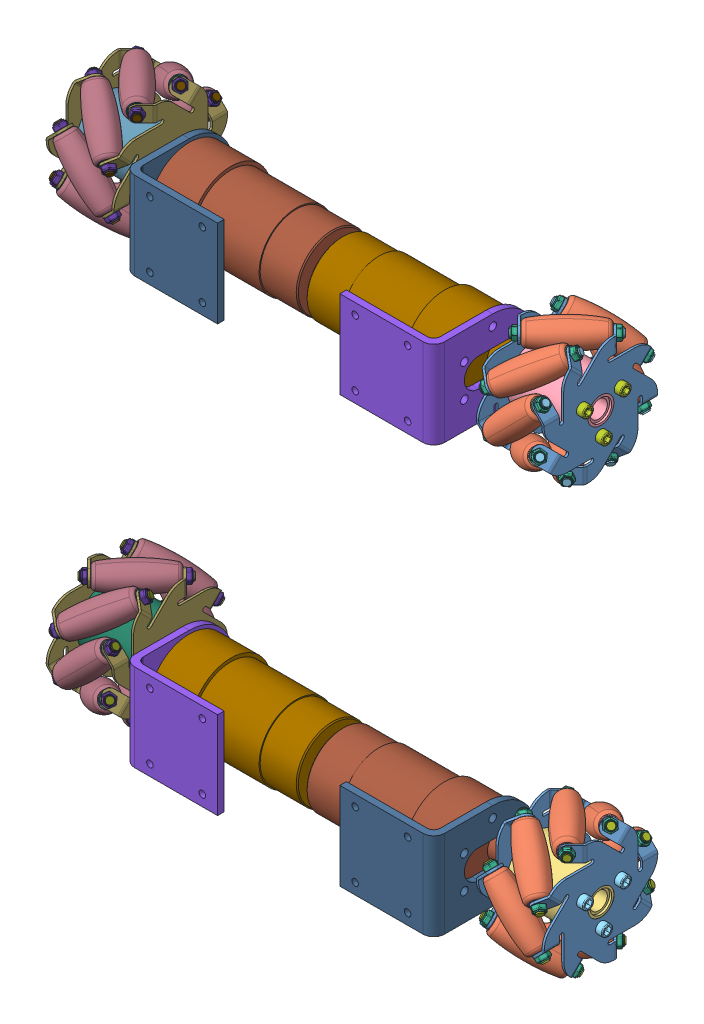
SolidWorks assembly car, configuration 默认. Lengths in mm.
Overall size (280 281.77 89.29).
257 component instances, 48 part files, 0 mates.
Components (placement in the parent):
- Tank(2)^car-1: Tank(2)^car [默认] at origin size (280 382.88 170.83) (virtual)
  - Mecanum_Wheel_60mm_Right_ASM_AP214 v1^Tank(2)_car-1: Mecanum_Wheel_60mm_Right_ASM_AP214 v1^Tank(2)_car [默认] at (62.5 -23.5276 -89.1195) x (1 0 0) z (0 0 -1) size (83 63.25 63.25) (virtual)
    - plate_2_Varsayilan^Mecanum_Wheel_60mm_Right_ASM_AP214 v1_Tank(2)_car-1: plate_2_Varsayilan^Mecanum_Wheel_60mm_Right_ASM_AP214 v1_Tank(2)_car [默认] at (56.8037 4.8798 97.2247) x (0.707107 0.707107 0) z (0 0 1) size (41.63 41.63 53.77) (virtual)
    - roller_Varsayilan^Mecanum_Wheel_60mm_Right_ASM_AP214 v1_Tank(2)_car-1: roller_Varsayilan^Mecanum_Wheel_60mm_Right_ASM_AP214 v1_Tank(2)_car [默认] at (15.1622 40.0059 51.0708) x (-0.707107 0.5 0.5) z (-0.704237 -0.434326 -0.561615) size (29.8 12.94 12.94) (virtual)
    - liner_Varsayilan^Mecanum_Wheel_60mm_Right_ASM_AP214 v1_Tank(2)_car-1: liner_Varsayilan^Mecanum_Wheel_60mm_Right_ASM_AP214 v1_Tank(2)_car [默认] at (4.8906 47.2689 58.3339) x (-0.663539 -0.224823 -0.713562) z (-0.24437 -0.836334 0.490743) size (7 1 7) (virtual)
    - inner_cylinder_Varsayilan^Mecanum_Wheel_60mm_Right_ASM_AP214 v1_Tank(2)_car-1: inner_cylinder_Varsayilan^Mecanum_Wheel_60mm_Right_ASM_AP214 v1_Tank(2)_car [默认] at (30 23.5276 67.1195) x (0 0 1) z (-1 0 0) size (26 26 31) (virtual)
    - two_sided_screw_Varsayilan^Mecanum_Wheel_60mm_Right_ASM_AP214 v1_Tank(2)_car-1: two_sided_screw_Varsayilan^Mecanum_Wheel_60mm_Right_ASM_AP214 v1_Tank(2)_car [默认] at (28.9323 30.2689 41.3339) x (-0.195015 0.541787 -0.817579) z (-0.707107 0.5 0.5) size (3 3 38) (virtual)
    - 3mm_bolt_Varsayilan^Mecanum_Wheel_60mm_Right_ASM_AP214 v1_Tank(2)_car-1: 3mm_bolt_Varsayilan^Mecanum_Wheel_60mm_Right_ASM_AP214 v1_Tank(2)_car [默认] at (4.155 47.7891 58.854) x (0.638071 0.755922 0.146447) z (-0.707107 0.5 0.5) size (5.6 5.2 2.5) (virtual)
    - 3x35_screw_Varsayilan^Mecanum_Wheel_60mm_Right_ASM_AP214 v1_Tank(2)_car-1: 3x35_screw_Varsayilan^Mecanum_Wheel_60mm_Right_ASM_AP214 v1_Tank(2)_car [默认] at (-3 18.5276 58.4592) x (0 0.745603 -0.666391) z (1 0 0) size (5 5 37) (virtual)
    - plate_2_Varsayilan^Mecanum_Wheel_60mm_Right_ASM_AP214 v1_Tank(2)_car-2: plate_2_Varsayilan^Mecanum_Wheel_60mm_Right_ASM_AP214 v1_Tank(2)_car [默认] at (-25.8037 4.8798 37.0142) x (-0.707107 0.707107 0) z (0 0 -1) size (41.63 41.63 53.77) (virtual)
    - liner_Varsayilan^Mecanum_Wheel_60mm_Right_ASM_AP214 v1_Tank(2)_car-2: liner_Varsayilan^Mecanum_Wheel_60mm_Right_ASM_AP214 v1_Tank(2)_car [默认] at (26.1038 32.2689 43.3339) x (0.54662 -0.062042 0.835079) z (-0.448561 -0.8638 0.22944) size (7 1 7) (virtual)
    - 3mm_bolt_Varsayilan^Mecanum_Wheel_60mm_Right_ASM_AP214 v1_Tank(2)_car-2: 3mm_bolt_Varsayilan^Mecanum_Wheel_60mm_Right_ASM_AP214 v1_Tank(2)_car [默认] at (26.8109 31.7689 42.8339) x (0.358192 -0.356391 0.862951) z (0.707107 -0.5 -0.5) size (5.6 5.2 2.5) (virtual)
    - 3mm_bolt_Varsayilan^Mecanum_Wheel_60mm_Right_ASM_AP214 v1_Tank(2)_car-3: 3mm_bolt_Varsayilan^Mecanum_Wheel_60mm_Right_ASM_AP214 v1_Tank(2)_car [默认] at (0 18.5276 75.7797) x (0 -0.80734 0.590087) z (-1 0 0) size (5.6 5.2 2.5) (virtual)
    - 3x35_screw_Varsayilan^Mecanum_Wheel_60mm_Right_ASM_AP214 v1_Tank(2)_car-2: 3x35_screw_Varsayilan^Mecanum_Wheel_60mm_Right_ASM_AP214 v1_Tank(2)_car [默认] at (-3 18.5276 75.7797) x (0 -0.949913 -0.312516) z (1 0 0) size (5 5 37) (virtual)
    - 3x35_screw_Varsayilan^Mecanum_Wheel_60mm_Right_ASM_AP214 v1_Tank(2)_car-3: 3x35_screw_Varsayilan^Mecanum_Wheel_60mm_Right_ASM_AP214 v1_Tank(2)_car [默认] at (-3 33.5276 67.1195) x (0 0.20431 0.978906) z (1 0 0) size (5 5 37) (virtual)
    - 3mm_bolt_Varsayilan^Mecanum_Wheel_60mm_Right_ASM_AP214 v1_Tank(2)_car-4: 3mm_bolt_Varsayilan^Mecanum_Wheel_60mm_Right_ASM_AP214 v1_Tank(2)_car [默认] at (0 33.5276 67.1195) x (0 0.9147 0.404133) z (-1 0 0) size (5.6 5.2 2.5) (virtual)
    - 3mm_bolt_Varsayilan^Mecanum_Wheel_60mm_Right_ASM_AP214 v1_Tank(2)_car-5: 3mm_bolt_Varsayilan^Mecanum_Wheel_60mm_Right_ASM_AP214 v1_Tank(2)_car [默认] at (0 18.5276 58.4592) x (0 -0.107361 -0.99422) z (-1 0 0) size (5.6 5.2 2.5) (virtual)
    - two_sided_screw_Varsayilan^Mecanum_Wheel_60mm_Right_ASM_AP214 v1_Tank(2)_car-2: two_sided_screw_Varsayilan^Mecanum_Wheel_60mm_Right_ASM_AP214 v1_Tank(2)_car [默认] at (28.9323 10.0613 44.1195) x (-0.195015 -0.195015 -0.961217) z (-0.707107 0.707107 0) size (3 3 38) (virtual)
    - two_sided_screw_Varsayilan^Mecanum_Wheel_60mm_Right_ASM_AP214 v1_Tank(2)_car-3: two_sided_screw_Varsayilan^Mecanum_Wheel_60mm_Right_ASM_AP214 v1_Tank(2)_car [默认] at (28.9323 -2.258 60.3781) x (-0.195015 -0.817579 -0.541787) z (-0.707107 0.5 -0.5) size (3 3 38) (virtual)
    - two_sided_screw_Varsayilan^Mecanum_Wheel_60mm_Right_ASM_AP214 v1_Tank(2)_car-4: two_sided_screw_Varsayilan^Mecanum_Wheel_60mm_Right_ASM_AP214 v1_Tank(2)_car [默认] at (28.9323 0.5276 80.5857) x (-0.195015 -0.961217 0.195015) z (-0.707107 0 -0.707107) size (3 3 38) (virtual)
    - two_sided_screw_Varsayilan^Mecanum_Wheel_60mm_Right_ASM_AP214 v1_Tank(2)_car-5: two_sided_screw_Varsayilan^Mecanum_Wheel_60mm_Right_ASM_AP214 v1_Tank(2)_car [默认] at (28.9323 16.7862 92.905) x (-0.195015 -0.541787 0.817579) z (-0.707107 -0.5 -0.5) size (3 3 38) (virtual)
    - two_sided_screw_Varsayilan^Mecanum_Wheel_60mm_Right_ASM_AP214 v1_Tank(2)_car-6: two_sided_screw_Varsayilan^Mecanum_Wheel_60mm_Right_ASM_AP214 v1_Tank(2)_car [默认] at (28.9323 36.9938 90.1195) x (-0.195015 0.195015 0.961217) z (-0.707107 -0.707107 0) size (3 3 38) (virtual)
    - two_sided_screw_Varsayilan^Mecanum_Wheel_60mm_Right_ASM_AP214 v1_Tank(2)_car-7: two_sided_screw_Varsayilan^Mecanum_Wheel_60mm_Right_ASM_AP214 v1_Tank(2)_car [默认] at (28.9323 49.3131 73.8608) x (-0.195015 0.817579 0.541787) z (-0.707107 -0.5 0.5) size (3 3 38) (virtual)
    - two_sided_screw_Varsayilan^Mecanum_Wheel_60mm_Right_ASM_AP214 v1_Tank(2)_car-8: two_sided_screw_Varsayilan^Mecanum_Wheel_60mm_Right_ASM_AP214 v1_Tank(2)_car [默认] at (28.9323 46.5276 53.6532) x (-0.195015 0.961217 -0.195015) z (-0.707107 0 0.707107) size (3 3 38) (virtual)
    - 3mm_bolt_Varsayilan^Mecanum_Wheel_60mm_Right_ASM_AP214 v1_Tank(2)_car-6: 3mm_bolt_Varsayilan^Mecanum_Wheel_60mm_Right_ASM_AP214 v1_Tank(2)_car [默认] at (26.8109 12.1826 44.1195) x (0.358192 0.358192 0.862205) z (0.707107 -0.707107 0) size (5.6 5.2 2.5) (virtual)
    - 3mm_bolt_Varsayilan^Mecanum_Wheel_60mm_Right_ASM_AP214 v1_Tank(2)_car-7: 3mm_bolt_Varsayilan^Mecanum_Wheel_60mm_Right_ASM_AP214 v1_Tank(2)_car [默认] at (26.8109 -0.758 58.8781) x (0.358192 0.862951 0.356391) z (0.707107 -0.5 0.5) size (5.6 5.2 2.5) (virtual)
    - 3mm_bolt_Varsayilan^Mecanum_Wheel_60mm_Right_ASM_AP214 v1_Tank(2)_car-8: 3mm_bolt_Varsayilan^Mecanum_Wheel_60mm_Right_ASM_AP214 v1_Tank(2)_car [默认] at (26.8109 0.5276 78.4644) x (0.358192 0.862205 -0.358192) z (0.707107 0 0.707107) size (5.6 5.2 2.5) (virtual)
    - 3mm_bolt_Varsayilan^Mecanum_Wheel_60mm_Right_ASM_AP214 v1_Tank(2)_car-9: 3mm_bolt_Varsayilan^Mecanum_Wheel_60mm_Right_ASM_AP214 v1_Tank(2)_car [默认] at (26.8109 15.2862 91.405) x (0.358192 0.356391 -0.862951) z (0.707107 0.5 0.5) size (5.6 5.2 2.5) (virtual)
    - 3mm_bolt_Varsayilan^Mecanum_Wheel_60mm_Right_ASM_AP214 v1_Tank(2)_car-10: 3mm_bolt_Varsayilan^Mecanum_Wheel_60mm_Right_ASM_AP214 v1_Tank(2)_car [默认] at (26.8109 34.8725 90.1195) x (0.358192 -0.358192 -0.862205) z (0.707107 0.707107 0) size (5.6 5.2 2.5) (virtual)
    - 3mm_bolt_Varsayilan^Mecanum_Wheel_60mm_Right_ASM_AP214 v1_Tank(2)_car-11: 3mm_bolt_Varsayilan^Mecanum_Wheel_60mm_Right_ASM_AP214 v1_Tank(2)_car [默认] at (26.8109 47.8131 75.3608) x (0.358192 -0.862951 -0.356391) z (0.707107 0.5 -0.5) size (5.6 5.2 2.5) (virtual)
    - 3mm_bolt_Varsayilan^Mecanum_Wheel_60mm_Right_ASM_AP214 v1_Tank(2)_car-12: 3mm_bolt_Varsayilan^Mecanum_Wheel_60mm_Right_ASM_AP214 v1_Tank(2)_car [默认] at (26.8109 46.5276 55.7745) x (0.358192 -0.862205 0.358192) z (0.707107 0 -0.707107) size (5.6 5.2 2.5) (virtual)
    - 3mm_bolt_Varsayilan^Mecanum_Wheel_60mm_Right_ASM_AP214 v1_Tank(2)_car-13: 3mm_bolt_Varsayilan^Mecanum_Wheel_60mm_Right_ASM_AP214 v1_Tank(2)_car [默认] at (4.155 34.8385 44.1195) x (0.638071 0.638071 -0.430964) z (-0.707107 0.707107 0) size (5.6 5.2 2.5) (virtual)
    - 3mm_bolt_Varsayilan^Mecanum_Wheel_60mm_Right_ASM_AP214 v1_Tank(2)_car-14: 3mm_bolt_Varsayilan^Mecanum_Wheel_60mm_Right_ASM_AP214 v1_Tank(2)_car [默认] at (4.155 15.2622 42.858) x (0.638071 0.146447 -0.755922) z (-0.707107 0.5 -0.5) size (5.6 5.2 2.5) (virtual)
    - 3mm_bolt_Varsayilan^Mecanum_Wheel_60mm_Right_ASM_AP214 v1_Tank(2)_car-15: 3mm_bolt_Varsayilan^Mecanum_Wheel_60mm_Right_ASM_AP214 v1_Tank(2)_car [默认] at (4.155 0.5276 55.8085) x (0.638071 -0.430964 -0.638071) z (-0.707107 0 -0.707107) size (5.6 5.2 2.5) (virtual)
    - 3mm_bolt_Varsayilan^Mecanum_Wheel_60mm_Right_ASM_AP214 v1_Tank(2)_car-16: 3mm_bolt_Varsayilan^Mecanum_Wheel_60mm_Right_ASM_AP214 v1_Tank(2)_car [默认] at (4.155 -0.7339 75.3849) x (0.638071 -0.755922 -0.146447) z (-0.707107 -0.5 -0.5) size (5.6 5.2 2.5) (virtual)
    - 3mm_bolt_Varsayilan^Mecanum_Wheel_60mm_Right_ASM_AP214 v1_Tank(2)_car-17: 3mm_bolt_Varsayilan^Mecanum_Wheel_60mm_Right_ASM_AP214 v1_Tank(2)_car [默认] at (4.155 12.2166 90.1195) x (0.638071 -0.638071 0.430964) z (-0.707107 -0.707107 0) size (5.6 5.2 2.5) (virtual)
    - 3mm_bolt_Varsayilan^Mecanum_Wheel_60mm_Right_ASM_AP214 v1_Tank(2)_car-18: 3mm_bolt_Varsayilan^Mecanum_Wheel_60mm_Right_ASM_AP214 v1_Tank(2)_car [默认] at (4.155 31.793 91.381) x (0.638071 -0.146447 0.755922) z (-0.707107 -0.5 0.5) size (5.6 5.2 2.5) (virtual)
    - 3mm_bolt_Varsayilan^Mecanum_Wheel_60mm_Right_ASM_AP214 v1_Tank(2)_car-19: 3mm_bolt_Varsayilan^Mecanum_Wheel_60mm_Right_ASM_AP214 v1_Tank(2)_car [默认] at (4.155 46.5276 78.4304) x (0.638071 0.430964 0.638071) z (-0.707107 0 0.707107) size (5.6 5.2 2.5) (virtual)
    - liner_Varsayilan^Mecanum_Wheel_60mm_Right_ASM_AP214 v1_Tank(2)_car-3: liner_Varsayilan^Mecanum_Wheel_60mm_Right_ASM_AP214 v1_Tank(2)_car [默认] at (26.1038 12.8897 44.1195) x (0.54662 0.54662 0.634361) z (-0.448561 -0.448561 0.773037) size (7 1 7) (virtual)
    - liner_Varsayilan^Mecanum_Wheel_60mm_Right_ASM_AP214 v1_Tank(2)_car-4: liner_Varsayilan^Mecanum_Wheel_60mm_Right_ASM_AP214 v1_Tank(2)_car [默认] at (26.1038 -0.258 58.3781) x (0.54662 0.835079 0.062042) z (-0.448561 0.22944 0.8638) size (7 1 7) (virtual)
    - liner_Varsayilan^Mecanum_Wheel_60mm_Right_ASM_AP214 v1_Tank(2)_car-5: liner_Varsayilan^Mecanum_Wheel_60mm_Right_ASM_AP214 v1_Tank(2)_car [默认] at (26.1038 0.5276 77.7573) x (0.54662 0.634361 -0.54662) z (-0.448561 0.773037 0.448561) size (7 1 7) (virtual)
    - liner_Varsayilan^Mecanum_Wheel_60mm_Right_ASM_AP214 v1_Tank(2)_car-6: liner_Varsayilan^Mecanum_Wheel_60mm_Right_ASM_AP214 v1_Tank(2)_car [默认] at (26.1038 14.7862 90.905) x (0.54662 0.062042 -0.835079) z (-0.448561 0.8638 -0.22944) size (7 1 7) (virtual)
    - liner_Varsayilan^Mecanum_Wheel_60mm_Right_ASM_AP214 v1_Tank(2)_car-7: liner_Varsayilan^Mecanum_Wheel_60mm_Right_ASM_AP214 v1_Tank(2)_car [默认] at (26.1038 34.1654 90.1195) x (0.54662 -0.54662 -0.634361) z (-0.448561 0.448561 -0.773037) size (7 1 7) (virtual)
    - liner_Varsayilan^Mecanum_Wheel_60mm_Right_ASM_AP214 v1_Tank(2)_car-8: liner_Varsayilan^Mecanum_Wheel_60mm_Right_ASM_AP214 v1_Tank(2)_car [默认] at (26.1038 47.3131 75.8608) x (0.54662 -0.835079 -0.062042) z (-0.448561 -0.22944 -0.8638) size (7 1 7) (virtual)
    - liner_Varsayilan^Mecanum_Wheel_60mm_Right_ASM_AP214 v1_Tank(2)_car-9: liner_Varsayilan^Mecanum_Wheel_60mm_Right_ASM_AP214 v1_Tank(2)_car [默认] at (26.1038 46.5276 56.4816) x (0.54662 -0.634361 0.54662) z (-0.448561 -0.773037 -0.448561) size (7 1 7) (virtual)
    - liner_Varsayilan^Mecanum_Wheel_60mm_Right_ASM_AP214 v1_Tank(2)_car-10: liner_Varsayilan^Mecanum_Wheel_60mm_Right_ASM_AP214 v1_Tank(2)_car [默认] at (4.8906 34.1029 44.1195) x (-0.663539 -0.663539 -0.345591) z (-0.24437 -0.24437 0.938385) size (7 1 7) (virtual)
    - liner_Varsayilan^Mecanum_Wheel_60mm_Right_ASM_AP214 v1_Tank(2)_car-11: liner_Varsayilan^Mecanum_Wheel_60mm_Right_ASM_AP214 v1_Tank(2)_car [默认] at (4.8906 14.742 43.3781) x (-0.663539 -0.713562 0.224823) z (-0.24437 0.490743 0.836334) size (7 1 7) (virtual)
    - liner_Varsayilan^Mecanum_Wheel_60mm_Right_ASM_AP214 v1_Tank(2)_car-12: liner_Varsayilan^Mecanum_Wheel_60mm_Right_ASM_AP214 v1_Tank(2)_car [默认] at (4.8906 0.5276 56.5441) x (-0.663539 -0.345591 0.663539) z (-0.24437 0.938385 0.24437) size (7 1 7) (virtual)
    - liner_Varsayilan^Mecanum_Wheel_60mm_Right_ASM_AP214 v1_Tank(2)_car-13: liner_Varsayilan^Mecanum_Wheel_60mm_Right_ASM_AP214 v1_Tank(2)_car [默认] at (4.8906 -0.2138 75.905) x (-0.663539 0.224823 0.713562) z (-0.24437 0.836334 -0.490743) size (7 1 7) (virtual)
    - liner_Varsayilan^Mecanum_Wheel_60mm_Right_ASM_AP214 v1_Tank(2)_car-14: liner_Varsayilan^Mecanum_Wheel_60mm_Right_ASM_AP214 v1_Tank(2)_car [默认] at (4.8906 12.9522 90.1195) x (-0.663539 0.663539 0.345591) z (-0.24437 0.24437 -0.938385) size (7 1 7) (virtual)
    - liner_Varsayilan^Mecanum_Wheel_60mm_Right_ASM_AP214 v1_Tank(2)_car-15: liner_Varsayilan^Mecanum_Wheel_60mm_Right_ASM_AP214 v1_Tank(2)_car [默认] at (4.8906 32.3131 90.8608) x (-0.663539 0.713562 -0.224823) z (-0.24437 -0.490743 -0.836334) size (7 1 7) (virtual)
    - liner_Varsayilan^Mecanum_Wheel_60mm_Right_ASM_AP214 v1_Tank(2)_car-16: liner_Varsayilan^Mecanum_Wheel_60mm_Right_ASM_AP214 v1_Tank(2)_car [默认] at (4.8906 46.5276 77.6948) x (-0.663539 0.345591 -0.663539) z (-0.24437 -0.938385 -0.24437) size (7 1 7) (virtual)
    - roller_Varsayilan^Mecanum_Wheel_60mm_Right_ASM_AP214 v1_Tank(2)_car-2: roller_Varsayilan^Mecanum_Wheel_60mm_Right_ASM_AP214 v1_Tank(2)_car [默认] at (15.1622 23.8314 44.1195) x (-0.707107 0.707107 0) z (-0.704237 -0.704237 -0.090007) size (29.8 12.94 12.94) (virtual)
    - roller_Varsayilan^Mecanum_Wheel_60mm_Right_ASM_AP214 v1_Tank(2)_car-3: roller_Varsayilan^Mecanum_Wheel_60mm_Right_ASM_AP214 v1_Tank(2)_car [默认] at (15.1622 7.4789 50.6412) x (-0.707107 0.5 -0.5) z (-0.704237 -0.561615 0.434326) size (29.8 12.94 12.94) (virtual)
    - roller_Varsayilan^Mecanum_Wheel_60mm_Right_ASM_AP214 v1_Tank(2)_car-4: roller_Varsayilan^Mecanum_Wheel_60mm_Right_ASM_AP214 v1_Tank(2)_car [默认] at (15.1622 0.5276 66.8156) x (-0.707107 0 -0.707107) z (-0.704237 -0.090007 0.704237) size (29.8 12.94 12.94) (virtual)
    - roller_Varsayilan^Mecanum_Wheel_60mm_Right_ASM_AP214 v1_Tank(2)_car-5: roller_Varsayilan^Mecanum_Wheel_60mm_Right_ASM_AP214 v1_Tank(2)_car [默认] at (15.1622 7.0493 83.1681) x (-0.707107 -0.5 -0.5) z (-0.704237 0.434326 0.561615) size (29.8 12.94 12.94) (virtual)
    - roller_Varsayilan^Mecanum_Wheel_60mm_Right_ASM_AP214 v1_Tank(2)_car-6: roller_Varsayilan^Mecanum_Wheel_60mm_Right_ASM_AP214 v1_Tank(2)_car [默认] at (15.1622 23.2237 90.1195) x (-0.707107 -0.707107 0) z (-0.704237 0.704237 0.090007) size (29.8 12.94 12.94) (virtual)
    - roller_Varsayilan^Mecanum_Wheel_60mm_Right_ASM_AP214 v1_Tank(2)_car-7: roller_Varsayilan^Mecanum_Wheel_60mm_Right_ASM_AP214 v1_Tank(2)_car [默认] at (15.1622 39.5762 83.5977) x (-0.707107 -0.5 0.5) z (-0.704237 0.561615 -0.434326) size (29.8 12.94 12.94) (virtual)
    - roller_Varsayilan^Mecanum_Wheel_60mm_Right_ASM_AP214 v1_Tank(2)_car-8: roller_Varsayilan^Mecanum_Wheel_60mm_Right_ASM_AP214 v1_Tank(2)_car [默认] at (15.1622 46.5276 67.4233) x (-0.707107 0 0.707107) z (-0.704237 0.090007 -0.704237) size (29.8 12.94 12.94) (virtual)
  - DC RF^Tank(2)_car-1: DC RF^Tank(2)_car [默认] at (0 -47.0551 -178.2389) x (1 0 0) z (0 0 -1) size (95 40 47) (virtual)
    - Component10^DC RF_Tank(2)_car-1: Component10^DC RF_Tank(2)_car [默认] at origin size (43 40 47) (virtual)
    - DC RF-0^DC RF_Tank(2)_car-1: DC RF-0^DC RF_Tank(2)_car [默认] at origin size (95 37 37) (virtual)
  - DC LF^Tank(2)_car-1: DC LF^Tank(2)_car [默认] at (-41 -47.0551 -178.2389) x (-1 0 0) z (0 0 1) size (95 40 47) (virtual)
    - Component10(Mirror)^DC LF_Tank(2)_car-1: Component10(Mirror)^DC LF_Tank(2)_car [默认] at origin size (43 40 47) (virtual)
    - DC LF-1^DC LF_Tank(2)_car-1: DC LF-1^DC LF_Tank(2)_car [默认] at origin size (95 37 37) (virtual)
  - Mecanum_Wheel_60mm_Left_ASM_AP214 v1^Tank(2)_car-1: Mecanum_Wheel_60mm_Left_ASM_AP214 v1^Tank(2)_car [默认] at (-107.4753 -26.4281 -134.5883) x (1 0 0) z (0 -0.707107 -0.707107) size (37 63.14 63.14) (virtual)
    - plate_1_Varsayilan^Mecanum_Wheel_60mm_Left_ASM_AP214 v1_Tank(2)_car-1: plate_1_Varsayilan^Mecanum_Wheel_60mm_Left_ASM_AP214 v1_Tank(2)_car [默认] at (-26.0247 -30.9199 60) size (7.04 53.75 53.75) (virtual)
    - roller_Varsayilan (1)^Mecanum_Wheel_60mm_Left_ASM_AP214 v1_Tank(2)_car-1: roller_Varsayilan (1)^Mecanum_Wheel_60mm_Left_ASM_AP214 v1_Tank(2)_car [默认] at (-11.1205 15.2872 46.4107) x (0.707107 -0.5 0.5) z (-0.228848 -0.830871 -0.50723) size (29.8 12.94 12.94) (virtual)
    - inner_cylinder_Varsayilan (1)^Mecanum_Wheel_60mm_Left_ASM_AP214 v1_Tank(2)_car-1: inner_cylinder_Varsayilan (1)^Mecanum_Wheel_60mm_Left_ASM_AP214 v1_Tank(2)_car [默认] at (-26.0247 -0.7238 29.8948) x (0 0.707107 -0.707107) z (1 0 0) size (26 26 31) (virtual)
    - liner_Varsayilan (1)^Mecanum_Wheel_60mm_Left_ASM_AP214 v1_Tank(2)_car-1: liner_Varsayilan (1)^Mecanum_Wheel_60mm_Left_ASM_AP214 v1_Tank(2)_car [默认] at (-0.849 8.0242 53.6738) x (0.666667 0.707107 -0.235702) z (-0.235702 0.5 0.833333) size (7 1 7) (virtual)
    - 3x35_screw_Varsayilan (1)^Mecanum_Wheel_60mm_Left_ASM_AP214 v1_Tank(2)_car-1: 3x35_screw_Varsayilan (1)^Mecanum_Wheel_60mm_Left_ASM_AP214 v1_Tank(2)_car [默认] at (-29.9304 6.3473 36.9659) x (0 0 -1) z (1 0 0) size (5 5 37) (virtual)
    - 3mm_bolt_Varsayilan (1)^Mecanum_Wheel_60mm_Left_ASM_AP214 v1_Tank(2)_car-1: 3mm_bolt_Varsayilan (1)^Mecanum_Wheel_60mm_Left_ASM_AP214 v1_Tank(2)_car [默认] at (-27.0247 1.8644 20.2355) x (0 0.765139 -0.643866) z (-1 0 0) size (5.6 5.2 2.5) (virtual)
    - two_sided_screw_Varsayilan (1)^Mecanum_Wheel_60mm_Left_ASM_AP214 v1_Tank(2)_car-1: two_sided_screw_Varsayilan (1)^Mecanum_Wheel_60mm_Left_ASM_AP214 v1_Tank(2)_car [默认] at (-24.8906 6.0552 4.1469) x (-0.576606 0.817021 -0.001578) z (0.707107 0.5 0.5) size (3 3 38) (virtual)
    - plate_1_Varsayilan^Mecanum_Wheel_60mm_Left_ASM_AP214 v1_Tank(2)_car-2: plate_1_Varsayilan^Mecanum_Wheel_60mm_Left_ASM_AP214 v1_Tank(2)_car [默认] at (3.0696 29.3814 -0.3013) x (-1 0 0) z (0 1 0) size (7.04 53.75 53.75) (virtual)
    - liner_Varsayilan (1)^Mecanum_Wheel_60mm_Left_ASM_AP214 v1_Tank(2)_car-2: liner_Varsayilan (1)^Mecanum_Wheel_60mm_Left_ASM_AP214 v1_Tank(2)_car [默认] at (-22.0622 23.0242 38.6738) x (0 -0.707107 -0.707107) z (-0.707107 -0.5 0.5) size (7 1 7) (virtual)
    - liner_Varsayilan (1)^Mecanum_Wheel_60mm_Left_ASM_AP214 v1_Tank(2)_car-3: liner_Varsayilan (1)^Mecanum_Wheel_60mm_Left_ASM_AP214 v1_Tank(2)_car [默认] at (-22.0622 22.2762 19.3102) x (0 -1 0) z (-0.707107 0 0.707107) size (7 1 7) (virtual)
    - liner_Varsayilan (1)^Mecanum_Wheel_60mm_Left_ASM_AP214 v1_Tank(2)_car-4: liner_Varsayilan (1)^Mecanum_Wheel_60mm_Left_ASM_AP214 v1_Tank(2)_car [默认] at (-22.0622 8.0552 6.1469) x (0 -0.707107 0.707107) z (-0.707107 0.5 0.5) size (7 1 7) (virtual)
    - liner_Varsayilan (1)^Mecanum_Wheel_60mm_Left_ASM_AP214 v1_Tank(2)_car-5: liner_Varsayilan (1)^Mecanum_Wheel_60mm_Left_ASM_AP214 v1_Tank(2)_car [默认] at (-22.0622 -11.3084 6.8948) x (0 0 1) z (-0.707107 0.707107 0) size (7 1 7) (virtual)
    - liner_Varsayilan (1)^Mecanum_Wheel_60mm_Left_ASM_AP214 v1_Tank(2)_car-6: liner_Varsayilan (1)^Mecanum_Wheel_60mm_Left_ASM_AP214 v1_Tank(2)_car [默认] at (-22.0622 -24.4717 21.1158) x (0 0.707107 0.707107) z (-0.707107 0.5 -0.5) size (7 1 7) (virtual)
    - liner_Varsayilan (1)^Mecanum_Wheel_60mm_Left_ASM_AP214 v1_Tank(2)_car-7: liner_Varsayilan (1)^Mecanum_Wheel_60mm_Left_ASM_AP214 v1_Tank(2)_car [默认] at (-22.0622 -23.7238 40.4794) x (0 1 0) z (-0.707107 0 -0.707107) size (7 1 7) (virtual)
    - liner_Varsayilan (1)^Mecanum_Wheel_60mm_Left_ASM_AP214 v1_Tank(2)_car-8: liner_Varsayilan (1)^Mecanum_Wheel_60mm_Left_ASM_AP214 v1_Tank(2)_car [默认] at (-22.0622 -9.5028 53.6427) x (0 0.707107 -0.707107) z (-0.707107 -0.5 -0.5) size (7 1 7) (virtual)
    - liner_Varsayilan (1)^Mecanum_Wheel_60mm_Left_ASM_AP214 v1_Tank(2)_car-9: liner_Varsayilan (1)^Mecanum_Wheel_60mm_Left_ASM_AP214 v1_Tank(2)_car [默认] at (-22.0622 9.8609 52.8948) x (0 0 -1) z (-0.707107 -0.707107 0) size (7 1 7) (virtual)
    - liner_Varsayilan (1)^Mecanum_Wheel_60mm_Left_ASM_AP214 v1_Tank(2)_car-10: liner_Varsayilan (1)^Mecanum_Wheel_60mm_Left_ASM_AP214 v1_Tank(2)_car [默认] at (-0.849 22.2762 40.5234) x (0.666667 0.333333 -0.666667) z (-0.235702 0.942809 0.235702) size (7 1 7) (virtual)
    - liner_Varsayilan (1)^Mecanum_Wheel_60mm_Left_ASM_AP214 v1_Tank(2)_car-11: liner_Varsayilan (1)^Mecanum_Wheel_60mm_Left_ASM_AP214 v1_Tank(2)_car [默认] at (-0.849 23.0552 21.1469) x (0.666667 -0.235702 -0.707107) z (-0.235702 0.833333 -0.5) size (7 1 7) (virtual)
    - liner_Varsayilan (1)^Mecanum_Wheel_60mm_Left_ASM_AP214 v1_Tank(2)_car-12: liner_Varsayilan (1)^Mecanum_Wheel_60mm_Left_ASM_AP214 v1_Tank(2)_car [默认] at (-0.849 9.9048 6.8948) x (0.666667 -0.666667 -0.333333) z (-0.235702 0.235702 -0.942809) size (7 1 7) (virtual)
    - liner_Varsayilan (1)^Mecanum_Wheel_60mm_Left_ASM_AP214 v1_Tank(2)_car-13: liner_Varsayilan (1)^Mecanum_Wheel_60mm_Left_ASM_AP214 v1_Tank(2)_car [默认] at (-0.849 -9.4717 6.1158) x (0.666667 -0.707107 0.235702) z (-0.235702 -0.5 -0.833333) size (7 1 7) (virtual)
    - liner_Varsayilan (1)^Mecanum_Wheel_60mm_Left_ASM_AP214 v1_Tank(2)_car-14: liner_Varsayilan (1)^Mecanum_Wheel_60mm_Left_ASM_AP214 v1_Tank(2)_car [默认] at (-0.849 -23.7238 19.2662) x (0.666667 -0.333333 0.666667) z (-0.235702 -0.942809 -0.235702) size (7 1 7) (virtual)
    - liner_Varsayilan (1)^Mecanum_Wheel_60mm_Left_ASM_AP214 v1_Tank(2)_car-15: liner_Varsayilan (1)^Mecanum_Wheel_60mm_Left_ASM_AP214 v1_Tank(2)_car [默认] at (-0.849 -24.5028 38.6427) x (0.666667 0.235702 0.707107) z (-0.235702 -0.833333 0.5) size (7 1 7) (virtual)
    - liner_Varsayilan (1)^Mecanum_Wheel_60mm_Left_ASM_AP214 v1_Tank(2)_car-16: liner_Varsayilan (1)^Mecanum_Wheel_60mm_Left_ASM_AP214 v1_Tank(2)_car [默认] at (-0.849 -11.3523 52.8948) x (0.666667 0.666667 0.333333) z (-0.235702 -0.235702 0.942809) size (7 1 7) (virtual)
    - roller_Varsayilan (1)^Mecanum_Wheel_60mm_Left_ASM_AP214 v1_Tank(2)_car-2: roller_Varsayilan (1)^Mecanum_Wheel_60mm_Left_ASM_AP214 v1_Tank(2)_car [默认] at (-11.1205 22.2762 30.2518) x (0.707107 0 0.707107) z (-0.228848 -0.94618 0.228848) size (29.8 12.94 12.94) (virtual)
    - roller_Varsayilan (1)^Mecanum_Wheel_60mm_Left_ASM_AP214 v1_Tank(2)_car-3: roller_Varsayilan (1)^Mecanum_Wheel_60mm_Left_ASM_AP214 v1_Tank(2)_car [默认] at (-11.1205 15.7922 13.8838) x (0.707107 0.5 0.5) z (-0.228848 -0.50723 0.830871) size (29.8 12.94 12.94) (virtual)
    - roller_Varsayilan (1)^Mecanum_Wheel_60mm_Left_ASM_AP214 v1_Tank(2)_car-4: roller_Varsayilan (1)^Mecanum_Wheel_60mm_Left_ASM_AP214 v1_Tank(2)_car [默认] at (-11.1205 -0.3667 6.8948) x (0.707107 0.707107 0) z (-0.228848 0.228848 0.94618) size (29.8 12.94 12.94) (virtual)
    - roller_Varsayilan (1)^Mecanum_Wheel_60mm_Left_ASM_AP214 v1_Tank(2)_car-5: roller_Varsayilan (1)^Mecanum_Wheel_60mm_Left_ASM_AP214 v1_Tank(2)_car [默认] at (-11.1205 -16.7348 13.3789) x (0.707107 0.5 -0.5) z (-0.228848 0.830871 0.50723) size (29.8 12.94 12.94) (virtual)
    - roller_Varsayilan (1)^Mecanum_Wheel_60mm_Left_ASM_AP214 v1_Tank(2)_car-6: roller_Varsayilan (1)^Mecanum_Wheel_60mm_Left_ASM_AP214 v1_Tank(2)_car [默认] at (-11.1205 -23.7238 29.5377) x (0.707107 0 -0.707107) z (-0.228848 0.94618 -0.228848) size (29.8 12.94 12.94) (virtual)
    - roller_Varsayilan (1)^Mecanum_Wheel_60mm_Left_ASM_AP214 v1_Tank(2)_car-7: roller_Varsayilan (1)^Mecanum_Wheel_60mm_Left_ASM_AP214 v1_Tank(2)_car [默认] at (-11.1205 -17.2397 45.9058) x (0.707107 -0.5 -0.5) z (-0.228848 0.50723 -0.830871) size (29.8 12.94 12.94) (virtual)
    - roller_Varsayilan (1)^Mecanum_Wheel_60mm_Left_ASM_AP214 v1_Tank(2)_car-8: roller_Varsayilan (1)^Mecanum_Wheel_60mm_Left_ASM_AP214 v1_Tank(2)_car [默认] at (-11.1205 -1.0808 52.8948) x (0.707107 -0.707107 0) z (-0.228848 -0.228848 -0.94618) size (29.8 12.94 12.94) (virtual)
    - 3x35_screw_Varsayilan (1)^Mecanum_Wheel_60mm_Left_ASM_AP214 v1_Tank(2)_car-2: 3x35_screw_Varsayilan (1)^Mecanum_Wheel_60mm_Left_ASM_AP214 v1_Tank(2)_car [默认] at (-29.9304 1.8644 20.2355) x (0 -0.866025 0.5) z (1 0 0) size (5 5 37) (virtual)
    - 3x35_screw_Varsayilan (1)^Mecanum_Wheel_60mm_Left_ASM_AP214 v1_Tank(2)_car-3: 3x35_screw_Varsayilan (1)^Mecanum_Wheel_60mm_Left_ASM_AP214 v1_Tank(2)_car [默认] at (-29.9304 -10.383 32.483) x (0 0.866025 0.5) z (1 0 0) size (5 5 37) (virtual)
    - 3mm_bolt_Varsayilan (1)^Mecanum_Wheel_60mm_Left_ASM_AP214 v1_Tank(2)_car-2: 3mm_bolt_Varsayilan (1)^Mecanum_Wheel_60mm_Left_ASM_AP214 v1_Tank(2)_car [默认] at (-27.0247 -10.383 32.483) x (0 -0.940173 -0.340697) z (-1 0 0) size (5.6 5.2 2.5) (virtual)
    - 3mm_bolt_Varsayilan (1)^Mecanum_Wheel_60mm_Left_ASM_AP214 v1_Tank(2)_car-3: 3mm_bolt_Varsayilan (1)^Mecanum_Wheel_60mm_Left_ASM_AP214 v1_Tank(2)_car [默认] at (-27.0247 6.3473 36.9659) x (0 0.175035 0.984562) z (-1 0 0) size (5.6 5.2 2.5) (virtual)
    - 3mm_bolt_Varsayilan (1)^Mecanum_Wheel_60mm_Left_ASM_AP214 v1_Tank(2)_car-4: 3mm_bolt_Varsayilan (1)^Mecanum_Wheel_60mm_Left_ASM_AP214 v1_Tank(2)_car [默认] at (-22.8133 7.5242 5.6158) x (-0.060636 0.747379 -0.661626) z (-0.707107 -0.5 -0.5) size (5.6 5.2 2.5) (virtual)
    - 3mm_bolt_Varsayilan (1)^Mecanum_Wheel_60mm_Left_ASM_AP214 v1_Tank(2)_car-5: 3mm_bolt_Varsayilan (1)^Mecanum_Wheel_60mm_Left_ASM_AP214 v1_Tank(2)_car [默认] at (-0.1419 23.5552 21.6469) x (0.267213 0.465725 -0.843622) z (0.707107 0.5 0.5) size (5.6 5.2 2.5) (virtual)
    - 3mm_bolt_Varsayilan (1)^Mecanum_Wheel_60mm_Left_ASM_AP214 v1_Tank(2)_car-6: 3mm_bolt_Varsayilan (1)^Mecanum_Wheel_60mm_Left_ASM_AP214 v1_Tank(2)_car [默认] at (-22.8133 22.2762 18.5591) x (-0.060636 0.996316 0.060636) z (-0.707107 0 -0.707107) size (5.6 5.2 2.5) (virtual)
    - 3mm_bolt_Varsayilan (1)^Mecanum_Wheel_60mm_Left_ASM_AP214 v1_Tank(2)_car-7: 3mm_bolt_Varsayilan (1)^Mecanum_Wheel_60mm_Left_ASM_AP214 v1_Tank(2)_car [默认] at (-22.8133 23.5552 38.1427) x (-0.060636 0.661626 0.747379) z (-0.707107 0.5 -0.5) size (5.6 5.2 2.5) (virtual)
    - 3mm_bolt_Varsayilan (1)^Mecanum_Wheel_60mm_Left_ASM_AP214 v1_Tank(2)_car-8: 3mm_bolt_Varsayilan (1)^Mecanum_Wheel_60mm_Left_ASM_AP214 v1_Tank(2)_car [默认] at (-22.8133 10.6119 52.8948) x (-0.060636 -0.060636 0.996316) z (-0.707107 0.707107 0) size (5.6 5.2 2.5) (virtual)
    - 3mm_bolt_Varsayilan (1)^Mecanum_Wheel_60mm_Left_ASM_AP214 v1_Tank(2)_car-9: 3mm_bolt_Varsayilan (1)^Mecanum_Wheel_60mm_Left_ASM_AP214 v1_Tank(2)_car [默认] at (-22.8133 -8.9717 54.1738) x (-0.060636 -0.747379 0.661626) z (-0.707107 0.5 0.5) size (5.6 5.2 2.5) (virtual)
    - 3mm_bolt_Varsayilan (1)^Mecanum_Wheel_60mm_Left_ASM_AP214 v1_Tank(2)_car-10: 3mm_bolt_Varsayilan (1)^Mecanum_Wheel_60mm_Left_ASM_AP214 v1_Tank(2)_car [默认] at (-22.8133 -23.7238 41.2305) x (-0.060636 -0.996316 -0.060636) z (-0.707107 0 0.707107) size (5.6 5.2 2.5) (virtual)
    - 3mm_bolt_Varsayilan (1)^Mecanum_Wheel_60mm_Left_ASM_AP214 v1_Tank(2)_car-11: 3mm_bolt_Varsayilan (1)^Mecanum_Wheel_60mm_Left_ASM_AP214 v1_Tank(2)_car [默认] at (-22.8133 -25.0028 21.6469) x (-0.060636 -0.661626 -0.747379) z (-0.707107 -0.5 0.5) size (5.6 5.2 2.5) (virtual)
    - 3mm_bolt_Varsayilan (1)^Mecanum_Wheel_60mm_Left_ASM_AP214 v1_Tank(2)_car-12: 3mm_bolt_Varsayilan (1)^Mecanum_Wheel_60mm_Left_ASM_AP214 v1_Tank(2)_car [默认] at (-22.8133 -12.0594 6.8948) x (-0.060636 0.060636 -0.996316) z (-0.707107 -0.707107 0) size (5.6 5.2 2.5) (virtual)
    - 3mm_bolt_Varsayilan (1)^Mecanum_Wheel_60mm_Left_ASM_AP214 v1_Tank(2)_car-13: 3mm_bolt_Varsayilan (1)^Mecanum_Wheel_60mm_Left_ASM_AP214 v1_Tank(2)_car [默认] at (-0.1419 22.2762 41.2305) x (0.267213 0.925848 -0.267213) z (0.707107 0 0.707107) size (5.6 5.2 2.5) (virtual)
    - 3mm_bolt_Varsayilan (1)^Mecanum_Wheel_60mm_Left_ASM_AP214 v1_Tank(2)_car-14: 3mm_bolt_Varsayilan (1)^Mecanum_Wheel_60mm_Left_ASM_AP214 v1_Tank(2)_car [默认] at (-0.1419 7.5242 54.1738) x (0.267213 0.843622 0.465725) z (0.707107 -0.5 0.5) size (5.6 5.2 2.5) (virtual)
    - 3mm_bolt_Varsayilan (1)^Mecanum_Wheel_60mm_Left_ASM_AP214 v1_Tank(2)_car-15: 3mm_bolt_Varsayilan (1)^Mecanum_Wheel_60mm_Left_ASM_AP214 v1_Tank(2)_car [默认] at (-0.1419 -12.0594 52.8948) x (0.267213 0.267213 0.925848) z (0.707107 -0.707107 0) size (5.6 5.2 2.5) (virtual)
    - 3mm_bolt_Varsayilan (1)^Mecanum_Wheel_60mm_Left_ASM_AP214 v1_Tank(2)_car-16: 3mm_bolt_Varsayilan (1)^Mecanum_Wheel_60mm_Left_ASM_AP214 v1_Tank(2)_car [默认] at (-0.1419 -25.0028 38.1427) x (0.267213 -0.465725 0.843622) z (0.707107 -0.5 -0.5) size (5.6 5.2 2.5) (virtual)
    - 3mm_bolt_Varsayilan (1)^Mecanum_Wheel_60mm_Left_ASM_AP214 v1_Tank(2)_car-17: 3mm_bolt_Varsayilan (1)^Mecanum_Wheel_60mm_Left_ASM_AP214 v1_Tank(2)_car [默认] at (-0.1419 -23.7238 18.5591) x (0.267213 -0.925848 0.267213) z (0.707107 0 -0.707107) size (5.6 5.2 2.5) (virtual)
    - 3mm_bolt_Varsayilan (1)^Mecanum_Wheel_60mm_Left_ASM_AP214 v1_Tank(2)_car-18: 3mm_bolt_Varsayilan (1)^Mecanum_Wheel_60mm_Left_ASM_AP214 v1_Tank(2)_car [默认] at (-0.1419 -8.9717 5.6158) x (0.267213 -0.843622 -0.465725) z (0.707107 0.5 -0.5) size (5.6 5.2 2.5) (virtual)
    - 3mm_bolt_Varsayilan (1)^Mecanum_Wheel_60mm_Left_ASM_AP214 v1_Tank(2)_car-19: 3mm_bolt_Varsayilan (1)^Mecanum_Wheel_60mm_Left_ASM_AP214 v1_Tank(2)_car [默认] at (-0.1419 10.6119 6.8948) x (0.267213 -0.267213 -0.925848) z (0.707107 0.707107 0) size (5.6 5.2 2.5) (virtual)
    - two_sided_screw_Varsayilan (1)^Mecanum_Wheel_60mm_Left_ASM_AP214 v1_Tank(2)_car-2: two_sided_screw_Varsayilan (1)^Mecanum_Wheel_60mm_Left_ASM_AP214 v1_Tank(2)_car [默认] at (-24.8906 22.2762 16.4817) x (-0.576606 0.578837 0.576606) z (0.707107 0 0.707107) size (3 3 38) (virtual)
    - two_sided_screw_Varsayilan (1)^Mecanum_Wheel_60mm_Left_ASM_AP214 v1_Tank(2)_car-3: two_sided_screw_Varsayilan (1)^Mecanum_Wheel_60mm_Left_ASM_AP214 v1_Tank(2)_car [默认] at (-24.8906 25.0242 36.6738) x (-0.576606 0.001578 0.817021) z (0.707107 -0.5 0.5) size (3 3 38) (virtual)
    - two_sided_screw_Varsayilan (1)^Mecanum_Wheel_60mm_Left_ASM_AP214 v1_Tank(2)_car-4: two_sided_screw_Varsayilan (1)^Mecanum_Wheel_60mm_Left_ASM_AP214 v1_Tank(2)_car [默认] at (-24.8906 12.6893 52.8948) x (-0.576606 -0.576606 0.578837) z (0.707107 -0.707107 0) size (3 3 38) (virtual)
    - two_sided_screw_Varsayilan (1)^Mecanum_Wheel_60mm_Left_ASM_AP214 v1_Tank(2)_car-5: two_sided_screw_Varsayilan (1)^Mecanum_Wheel_60mm_Left_ASM_AP214 v1_Tank(2)_car [默认] at (-24.8906 -7.5028 55.6427) x (-0.576606 -0.817021 0.001578) z (0.707107 -0.5 -0.5) size (3 3 38) (virtual)
    - two_sided_screw_Varsayilan (1)^Mecanum_Wheel_60mm_Left_ASM_AP214 v1_Tank(2)_car-6: two_sided_screw_Varsayilan (1)^Mecanum_Wheel_60mm_Left_ASM_AP214 v1_Tank(2)_car [默认] at (-24.8906 -23.7238 43.3078) x (-0.576606 -0.578837 -0.576606) z (0.707107 0 -0.707107) size (3 3 38) (virtual)
    - two_sided_screw_Varsayilan (1)^Mecanum_Wheel_60mm_Left_ASM_AP214 v1_Tank(2)_car-7: two_sided_screw_Varsayilan (1)^Mecanum_Wheel_60mm_Left_ASM_AP214 v1_Tank(2)_car [默认] at (-24.8906 -26.4717 23.1158) x (-0.576606 -0.001578 -0.817021) z (0.707107 0.5 -0.5) size (3 3 38) (virtual)
    - two_sided_screw_Varsayilan (1)^Mecanum_Wheel_60mm_Left_ASM_AP214 v1_Tank(2)_car-8: two_sided_screw_Varsayilan (1)^Mecanum_Wheel_60mm_Left_ASM_AP214 v1_Tank(2)_car [默认] at (-24.8906 -14.1368 6.8948) x (-0.576606 0.576606 -0.578837) z (0.707107 0.707107 0) size (3 3 38) (virtual)
  - Mecanum_Wheel_60mm_Left_ASM_AP214 v1 (1)^Tank(2)_car-1: Mecanum_Wheel_60mm_Left_ASM_AP214 v1 (1)^Tank(2)_car [默认] at (89.5247 -221.4281 -134.5883) x (1 0 0) z (0 -0.707107 -0.707107) size (37 63.14 63.14) (virtual)
    - plate_1_Varsayilan^Mecanum_Wheel_60mm_Left_ASM_AP214 v1 (1)_Tank(2)_car-1: plate_1_Varsayilan^Mecanum_Wheel_60mm_Left_ASM_AP214 v1 (1)_Tank(2)_car [默认] at (-26.0247 -30.9199 60) size (7.04 53.75 53.75) (virtual)
    - roller_Varsayilan (1)^Mecanum_Wheel_60mm_Left_ASM_AP214 v1 (1)_Tank(2)_car-1: roller_Varsayilan (1)^Mecanum_Wheel_60mm_Left_ASM_AP214 v1 (1)_Tank(2)_car [默认] at (-11.1205 15.2872 46.4107) x (0.707107 -0.5 0.5) z (-0.228848 -0.830871 -0.50723) size (29.8 12.94 12.94) (virtual)
    - inner_cylinder_Varsayilan (1)^Mecanum_Wheel_60mm_Left_ASM_AP214 v1 (1)_Tank(2)_car-1: inner_cylinder_Varsayilan (1)^Mecanum_Wheel_60mm_Left_ASM_AP214 v1 (1)_Tank(2)_car [默认] at (-26.0247 -0.7238 29.8948) x (0 0.707107 -0.707107) z (1 0 0) size (26 26 31) (virtual)
    - liner_Varsayilan (1)^Mecanum_Wheel_60mm_Left_ASM_AP214 v1 (1)_Tank(2)_car-1: liner_Varsayilan (1)^Mecanum_Wheel_60mm_Left_ASM_AP214 v1 (1)_Tank(2)_car [默认] at (-0.849 8.0242 53.6738) x (0.666667 0.707107 -0.235702) z (-0.235702 0.5 0.833333) size (7 1 7) (virtual)
    - 3x35_screw_Varsayilan (1)^Mecanum_Wheel_60mm_Left_ASM_AP214 v1 (1)_Tank(2)_car-1: 3x35_screw_Varsayilan (1)^Mecanum_Wheel_60mm_Left_ASM_AP214 v1 (1)_Tank(2)_car [默认] at (-29.9304 6.3473 36.9659) x (0 0 -1) z (1 0 0) size (5 5 37) (virtual)
    - 3mm_bolt_Varsayilan (1)^Mecanum_Wheel_60mm_Left_ASM_AP214 v1 (1)_Tank(2)_car-1: 3mm_bolt_Varsayilan (1)^Mecanum_Wheel_60mm_Left_ASM_AP214 v1 (1)_Tank(2)_car [默认] at (-27.0247 1.8644 20.2355) x (0 0.765139 -0.643866) z (-1 0 0) size (5.6 5.2 2.5) (virtual)
    - two_sided_screw_Varsayilan (1)^Mecanum_Wheel_60mm_Left_ASM_AP214 v1 (1)_Tank(2)_car-1: two_sided_screw_Varsayilan (1)^Mecanum_Wheel_60mm_Left_ASM_AP214 v1 (1)_Tank(2)_car [默认] at (-24.8906 6.0552 4.1469) x (-0.576606 0.817021 -0.001578) z (0.707107 0.5 0.5) size (3 3 38) (virtual)
    - plate_1_Varsayilan^Mecanum_Wheel_60mm_Left_ASM_AP214 v1 (1)_Tank(2)_car-2: plate_1_Varsayilan^Mecanum_Wheel_60mm_Left_ASM_AP214 v1 (1)_Tank(2)_car [默认] at (3.0696 29.3814 -0.3013) x (-1 0 0) z (0 1 0) size (7.04 53.75 53.75) (virtual)
    - liner_Varsayilan (1)^Mecanum_Wheel_60mm_Left_ASM_AP214 v1 (1)_Tank(2)_car-2: liner_Varsayilan (1)^Mecanum_Wheel_60mm_Left_ASM_AP214 v1 (1)_Tank(2)_car [默认] at (-22.0622 23.0242 38.6738) x (0 -0.707107 -0.707107) z (-0.707107 -0.5 0.5) size (7 1 7) (virtual)
    - liner_Varsayilan (1)^Mecanum_Wheel_60mm_Left_ASM_AP214 v1 (1)_Tank(2)_car-3: liner_Varsayilan (1)^Mecanum_Wheel_60mm_Left_ASM_AP214 v1 (1)_Tank(2)_car [默认] at (-22.0622 22.2762 19.3102) x (0 -1 0) z (-0.707107 0 0.707107) size (7 1 7) (virtual)
    - liner_Varsayilan (1)^Mecanum_Wheel_60mm_Left_ASM_AP214 v1 (1)_Tank(2)_car-4: liner_Varsayilan (1)^Mecanum_Wheel_60mm_Left_ASM_AP214 v1 (1)_Tank(2)_car [默认] at (-22.0622 8.0552 6.1469) x (0 -0.707107 0.707107) z (-0.707107 0.5 0.5) size (7 1 7) (virtual)
    - liner_Varsayilan (1)^Mecanum_Wheel_60mm_Left_ASM_AP214 v1 (1)_Tank(2)_car-5: liner_Varsayilan (1)^Mecanum_Wheel_60mm_Left_ASM_AP214 v1 (1)_Tank(2)_car [默认] at (-22.0622 -11.3084 6.8948) x (0 0 1) z (-0.707107 0.707107 0) size (7 1 7) (virtual)
    - liner_Varsayilan (1)^Mecanum_Wheel_60mm_Left_ASM_AP214 v1 (1)_Tank(2)_car-6: liner_Varsayilan (1)^Mecanum_Wheel_60mm_Left_ASM_AP214 v1 (1)_Tank(2)_car [默认] at (-22.0622 -24.4717 21.1158) x (0 0.707107 0.707107) z (-0.707107 0.5 -0.5) size (7 1 7) (virtual)
    - liner_Varsayilan (1)^Mecanum_Wheel_60mm_Left_ASM_AP214 v1 (1)_Tank(2)_car-7: liner_Varsayilan (1)^Mecanum_Wheel_60mm_Left_ASM_AP214 v1 (1)_Tank(2)_car [默认] at (-22.0622 -23.7238 40.4794) x (0 1 0) z (-0.707107 0 -0.707107) size (7 1 7) (virtual)
    - liner_Varsayilan (1)^Mecanum_Wheel_60mm_Left_ASM_AP214 v1 (1)_Tank(2)_car-8: liner_Varsayilan (1)^Mecanum_Wheel_60mm_Left_ASM_AP214 v1 (1)_Tank(2)_car [默认] at (-22.0622 -9.5028 53.6427) x (0 0.707107 -0.707107) z (-0.707107 -0.5 -0.5) size (7 1 7) (virtual)
    - liner_Varsayilan (1)^Mecanum_Wheel_60mm_Left_ASM_AP214 v1 (1)_Tank(2)_car-9: liner_Varsayilan (1)^Mecanum_Wheel_60mm_Left_ASM_AP214 v1 (1)_Tank(2)_car [默认] at (-22.0622 9.8609 52.8948) x (0 0 -1) z (-0.707107 -0.707107 0) size (7 1 7) (virtual)
    - liner_Varsayilan (1)^Mecanum_Wheel_60mm_Left_ASM_AP214 v1 (1)_Tank(2)_car-10: liner_Varsayilan (1)^Mecanum_Wheel_60mm_Left_ASM_AP214 v1 (1)_Tank(2)_car [默认] at (-0.849 22.2762 40.5234) x (0.666667 0.333333 -0.666667) z (-0.235702 0.942809 0.235702) size (7 1 7) (virtual)
    - liner_Varsayilan (1)^Mecanum_Wheel_60mm_Left_ASM_AP214 v1 (1)_Tank(2)_car-11: liner_Varsayilan (1)^Mecanum_Wheel_60mm_Left_ASM_AP214 v1 (1)_Tank(2)_car [默认] at (-0.849 23.0552 21.1469) x (0.666667 -0.235702 -0.707107) z (-0.235702 0.833333 -0.5) size (7 1 7) (virtual)
    - liner_Varsayilan (1)^Mecanum_Wheel_60mm_Left_ASM_AP214 v1 (1)_Tank(2)_car-12: liner_Varsayilan (1)^Mecanum_Wheel_60mm_Left_ASM_AP214 v1 (1)_Tank(2)_car [默认] at (-0.849 9.9048 6.8948) x (0.666667 -0.666667 -0.333333) z (-0.235702 0.235702 -0.942809) size (7 1 7) (virtual)
    - liner_Varsayilan (1)^Mecanum_Wheel_60mm_Left_ASM_AP214 v1 (1)_Tank(2)_car-13: liner_Varsayilan (1)^Mecanum_Wheel_60mm_Left_ASM_AP214 v1 (1)_Tank(2)_car [默认] at (-0.849 -9.4717 6.1158) x (0.666667 -0.707107 0.235702) z (-0.235702 -0.5 -0.833333) size (7 1 7) (virtual)
    - liner_Varsayilan (1)^Mecanum_Wheel_60mm_Left_ASM_AP214 v1 (1)_Tank(2)_car-14: liner_Varsayilan (1)^Mecanum_Wheel_60mm_Left_ASM_AP214 v1 (1)_Tank(2)_car [默认] at (-0.849 -23.7238 19.2662) x (0.666667 -0.333333 0.666667) z (-0.235702 -0.942809 -0.235702) size (7 1 7) (virtual)
    - liner_Varsayilan (1)^Mecanum_Wheel_60mm_Left_ASM_AP214 v1 (1)_Tank(2)_car-15: liner_Varsayilan (1)^Mecanum_Wheel_60mm_Left_ASM_AP214 v1 (1)_Tank(2)_car [默认] at (-0.849 -24.5028 38.6427) x (0.666667 0.235702 0.707107) z (-0.235702 -0.833333 0.5) size (7 1 7) (virtual)
    - liner_Varsayilan (1)^Mecanum_Wheel_60mm_Left_ASM_AP214 v1 (1)_Tank(2)_car-16: liner_Varsayilan (1)^Mecanum_Wheel_60mm_Left_ASM_AP214 v1 (1)_Tank(2)_car [默认] at (-0.849 -11.3523 52.8948) x (0.666667 0.666667 0.333333) z (-0.235702 -0.235702 0.942809) size (7 1 7) (virtual)
